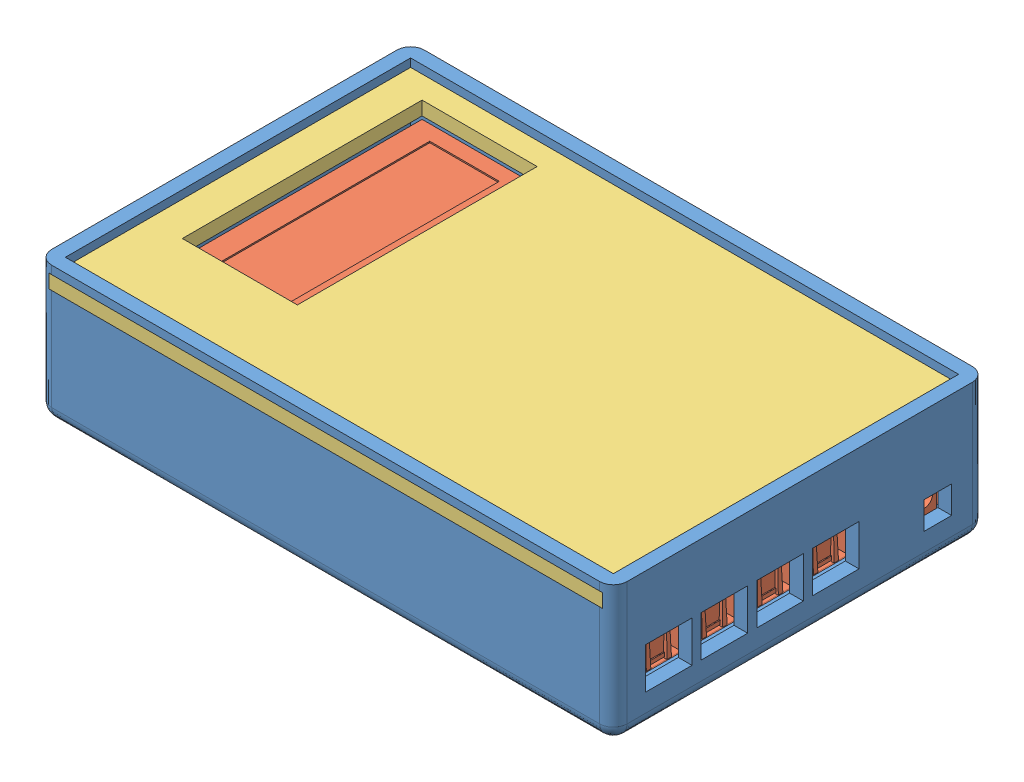
SolidWorks assembly Smarthome Case, configuration Default. Lengths in mm.
Overall size (210 50 136).
3 component instances, 3 part files, 5 mates.
Components (placement in the parent):
- Case 2-1: Case 2 [Default] at (-102.6374 -34.7797 69.3275) size (210 50 136)
- GSM-LCD-ATmega32_1-1: GSM-LCD-ATmega32_1 [Default] at (-102.2903 -24.3682 63.9775) x (1 0 0) z (0 1 0) size (199.65 120.89 39)
- Nap Case 2-2: Nap Case 2 [Default] at (-103.6374 7.2203 74.3275) size (202 5 133)
Mates (geometry in assembly coordinates):
- Distance1: distance = 5 mm anti-aligned: plane of Case 2-1 through (-102.6374 -29.7797 69.3275) normal (0 1 0); plane of GSM-LCD-ATmega32_1-1 through (-102.2903 -24.7797 63.9775) normal (0 -1 0)
- Coincident18: coincident anti-aligned: plane of Case 2-1 through (-102.6374 15.2203 -56.6725) normal (0 0 1); plane of GSM-LCD-ATmega32_1-1 through (94.5597 -24.7797 -56.6725) normal (0 0 -1)
- Coincident19: coincident anti-aligned: plane of Case 2-1 through (-103.6374 12.2203 -58.6725) normal (0 -1 0); plane of Nap Case 2-2 through (-103.6374 12.2203 74.3275) normal (0 1 0)
- Coincident20: coincident anti-aligned: plane of Case 2-1 through (98.3626 12.2203 -58.6725) normal (-1 0 0); plane of Nap Case 2-2 through (98.3626 12.2203 74.3275) normal (1 0 0)
- Coincident21: coincident aligned: plane of Case 2-1 through (-102.6374 15.2203 74.3275) normal (0 0 1); plane of Nap Case 2-2 through (-103.6374 12.2203 74.3275) normal (0 0 1)
